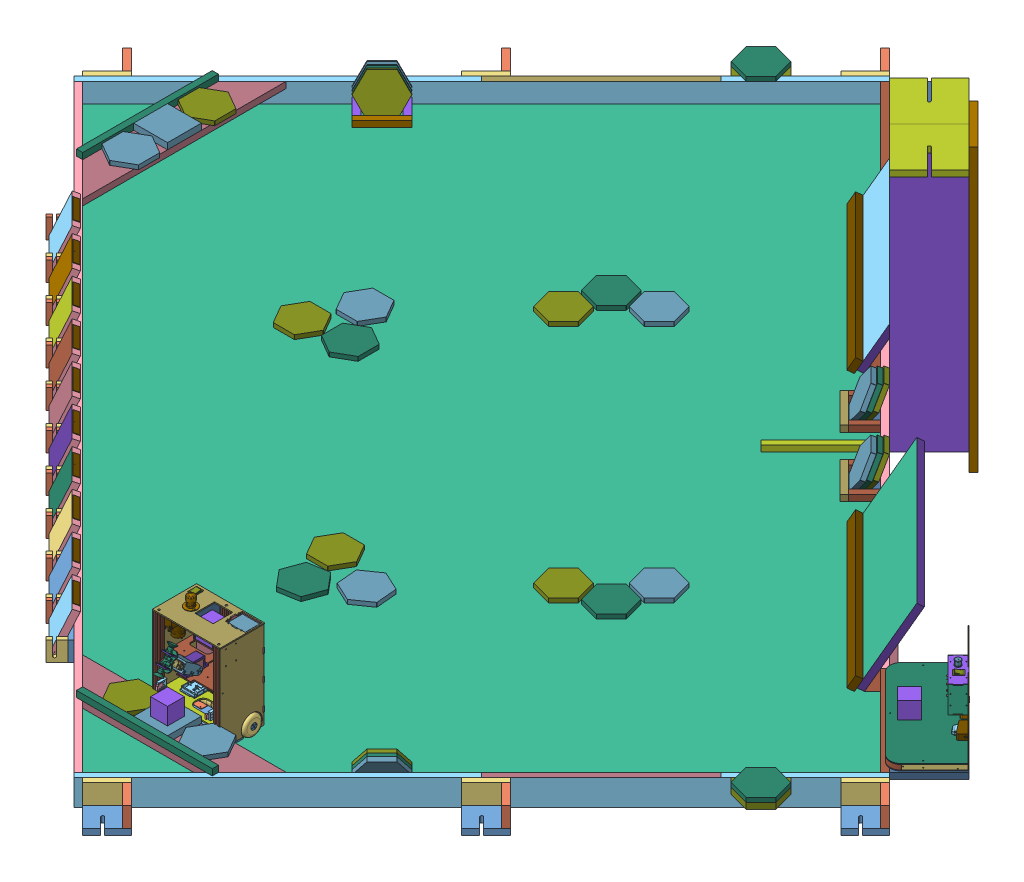
SolidWorks assembly conception_final_robot_autonome, configuration Default. Lengths in mm.
Overall size (3970.07 1029.4 3970.11).
442 component instances, 151 part files, 123 mates.
Components (placement in the parent):
- robot_sghyr-1: robot_sghyr [Default] at (76.8159 -4.9036 482.9829) x (0 0 1) z (0 1 0) size (182.75 247 90.25) (flexible)
  - base_robot_sghyr-1: base_robot_sghyr [Default] at (64.264 97.0127 214.7631) size (170 240 5)
  - 37 mm DC Geared Motor Mounting Bracket-1: 37 mm DC Geared Motor Mounting Bracket [Default] at (24.264 177.0127 247.7631) x (0 -1 0) z (-1 0 0) size (41 48 40)
  - pololu-37D-encoder-1: pololu-37D-encoder [Default] at (24.264 151.2127 247.7631) x (0 0 -1) z (0 1 0) size (36.8 36.8 92.61)
  - Robot2015_support bille porteuse-1: Robot2015_support bille porteuse [Défaut] at (126.764 97.0127 219.7631) x (-0.866025 -0.5 0) z (-0.5 0.866025 0) size (49.64 16.2 45)
  - 37 mm DC Geared Motor Mounting Bracket-3: 37 mm DC Geared Motor Mounting Bracket [Default] at (24.264 17.0127 247.7631) x (0 1 0) z (1 0 0) size (41 48 40)
  - pololu-37D-encoder-4: pololu-37D-encoder [Default] at (24.264 42.8127 247.7631) x (0 0 -1) z (0 -1 0) size (36.8 36.8 92.61)
  - Arduino Mega 2560.step-1: Arduino Mega 2560.step [Default] at (36.414 47.7209 283.4141) x (-1 0 0) z (0 0 -1) size (107.95 53.42 12.95)
  - Roulement_d3xd10xe4-1: Roulement_d3xd10xe4 [Défaut] at (146.264 -19.9873 225.0631) x (0 0 1) z (-1 0 0) size (5 13 13)
  - etage electronique-1: etage electronique [Default] at (64.264 97.0127 277.7631) x (0 -1 0) z (0 0 1) size (232 153 4)
  - XL4016E1 8A Buck Converter.STEP-1: XL4016E1 8A Buck Converter.STEP [Default] at (36.914 174.7627 281.7631) x (1 0 0) z (0 -1 0) size (65.3 28.6 46.4)
    - 8A Buck Converter PCB.STEP-1: 8A Buck Converter PCB.STEP [Default] at origin size (65.3 1.67 36.5)
    - Heat Exchanger.STEP-1: Heat Exchanger.STEP [Default] at (0 1.65 23.2) size (46 25.1 10.55)
    - Heat Exchanger.STEP-2: Heat Exchanger.STEP [Default] at (0 1.65 -23.2) x (-1 0 0) z (0 0 -1) size (46 25.1 10.55)
    - LargeGreen1000uF 35V Electrolytic Capacitor.STEP-1: LargeGreen1000uF 35V Electrolytic Capacitor.STEP [Default] at (-17.6782 1.65 7.8366) x (0 0 -1) z (1 0 0) size (9.9 26.01 9.9)
    - LargeGreen1000uF 35V Electrolytic Capacitor.STEP-2: LargeGreen1000uF 35V Electrolytic Capacitor.STEP [Default] at (-8.0317 1.65 5.0694) x (0 0 -1) z (1 0 0) size (9.9 26.01 9.9)
    - LargeGreen470uF 35V Electrolytic Capacitor.STEP-1: LargeGreen470uF 35V Electrolytic Capacitor.STEP [Default] at (-17.6617 1.65 -7.7514) x (0 0 1) z (-1 0 0) size (9.9 26.01 9.9)
    - LargeGreen470uF 35V Electrolytic Capacitor.STEP-2: LargeGreen470uF 35V Electrolytic Capacitor.STEP [Default] at (-7.9869 1.65 -5.0151) x (0 0 1) z (-1 0 0) size (9.9 26.01 9.9)
    - Screw Terminal x2.STEP-1: Screw Terminal x2.STEP [Default] at (-9.5 0 12.7839) x (-1 0 0) z (0 0 -1) size (7.95 12.9 10)
    - Screw Terminal x2.STEP-2: Screw Terminal x2.STEP [Default] at (-9.5 0 2.7839) x (-1 0 0) z (0 0 -1) size (7.95 12.9 10)
    - TrimmerW103.STEP-1: TrimmerW103.STEP [Default] at (32.65 6.9 -4.9563) x (0 0 1) z (-1 0 0) size (9.5 15.15 4.8)
    - TrimmerW103.STEP-2: TrimmerW103.STEP [Default] at (32.65 6.9 5.0581) x (0 0 1) z (-1 0 0) size (9.5 15.15 4.8)
    - whiteLEDShortLeed.STEP-1: whiteLEDShortLeed.STEP [Default] at (-13.9989 2.65 -0.1564) x (-1 0 0) z (0 0 -1) size (3.4 13.35 3.4)
    - Schottky Diode 20A 45V STPS2045CT.STEP-1: Schottky Diode 20A 45V STPS2045CT.STEP [Default] at (-0.0419 13.7002 12.65) x (-0.999962 0.008727 0) z (-0.008727 -0.999962 0) size (10.22 3.95 22.6)
    - XL4016E1 8A Voltage Regulator.STEP-1: XL4016E1 8A Voltage Regulator.STEP [Default] at (0 13.7 -12.65) x (1 0 0) z (0 -1 0) size (10.22 3.95 22.6)
    - Coil for Convertor.STEP-1: Coil for Convertor.STEP [Default] at (14.3115 2.9157 0.0112) size (27.99 14.39 26.86)
    - Small Plastic Washer.STEP-1: Small Plastic Washer.STEP [Default] at (0 18.5 -11.95) x (1 0 0) z (0 -1 0) size (6.1 1 6.1)
    - Small Plastic Washer.STEP-2: Small Plastic Washer.STEP [Default] at (0 18.5 10.95) x (1 0 0) z (0 -1 0) size (6.1 1 6.1)
    - pan head cross recess screw_iso_ISO 7045 - M3 x 8 - Z - 8S.STEP-1: pan head cross recess screw_iso_ISO 7045 - M3 x 8 - Z - 8S.STEP [Default] at (0 18.5 -8.55) x (0 0 -1) z (0.923728 0.383049 0) size (10.36 5.6 5.6)
    - pan head cross recess screw_iso_ISO 7045 - M3 x 8 - Z - 8S.STEP-2: pan head cross recess screw_iso_ISO 7045 - M3 x 8 - Z - 8S.STEP [Default] at (0 18.5 8.55) x (0 0 1) z (-1 0 0) size (10.36 5.6 5.6)
    - 1.7mmSmdCeramicCapacitorbrown.STEP-1: 1.7mmSmdCeramicCapacitorbrown.STEP [Default] at (2.849 0.0574 -8.3522) x (-1 0 0) z (0 0 1) size (2.02 0.49 1.04)
    - smdChip8pin.STEP-1: smdChip8pin.STEP [Default] at (19.9049 -0.725 7.6791) x (1 0 0) z (0 0 -1) size (7.3 1.22 4.5)
    - tinyVoltageRegulator.STEP-1: tinyVoltageRegulator.STEP [Default] at (13.3487 0 4.1964) x (-1 0 0) z (0 0 1) size (2.75 0.7 2.1)
    - tinyVoltageRegulator.STEP-2: tinyVoltageRegulator.STEP [Default] at (20.3011 0 11.2685) x (0.999962 0 0.008727) z (0.008727 0 -0.999962) size (2.75 0.7 2.1)
    - TinyVoltageRegulatorAMS1112.STEP-1: TinyVoltageRegulatorAMS1112.STEP [Default] at (15.0739 0.203 -4.8321) x (0 0 -1) z (-1 0 0) size (4.07 1.22 4.96)
    - tinySMDResistor222.STEP-1: tinySMDResistor222.STEP [Default] at (21.8501 0.1177 -6.1765) x (0 0 -1) z (-1 0 0) size (1.52 0.38 0.79)
    - tinySMDResistor.STEP-1: tinySMDResistor.STEP [Default] at (19.9225 0.1177 -6.1853) x (0 0 -1) z (-1 0 0) size (1.52 0.37 0.79)
    - 1.7mmSmdCeramicCapacitorbrown.STEP-2: 1.7mmSmdCeramicCapacitorbrown.STEP [Default] at (24.1073 0.0574 -6.3061) x (0 0 -1) z (-1 0 0) size (2.02 0.49 1.04)
    - 1.7mmSmdCeramicCapacitorbrown.STEP-3: 1.7mmSmdCeramicCapacitorbrown.STEP [Default] at (16.3262 0.0574 0.9562) x (0 0 -1) z (-1 0 0) size (2.02 0.49 1.04)
    - 1.7mmSmdCeramicCapacitorbrown.STEP-4: 1.7mmSmdCeramicCapacitorbrown.STEP [Default] at (18.1093 0.0574 0.9562) x (0 0 -1) z (-1 0 0) size (2.02 0.49 1.04)
    - tinySMDResistor.STEP-2: tinySMDResistor.STEP [Default] at (19.9874 0.1177 1.1419) x (0 0 -1) z (-1 0 0) size (1.52 0.37 0.79)
    - tinySMDResistor.STEP-3: tinySMDResistor.STEP [Default] at (21.6733 0.1177 1.1419) x (0 0 -1) z (-1 0 0) size (1.52 0.37 0.79)
    - tinySMDResistor.STEP-4: tinySMDResistor.STEP [Default] at (23.3916 0.1177 1.1419) x (0 0 -1) z (-1 0 0) size (1.52 0.37 0.79)
    - 1.7mmSmdCeramicCapacitorbrown.STEP-5: 1.7mmSmdCeramicCapacitorbrown.STEP [Default] at (25.4211 0.0574 4.0139) x (0 0 -1) z (-1 0 0) size (2.02 0.49 1.04)
    - 1.7mmSmdCeramicCapacitorbrown.STEP-6: 1.7mmSmdCeramicCapacitorbrown.STEP [Default] at (27.3088 0.0574 4.0139) x (0 0 -1) z (-1 0 0) size (2.02 0.49 1.04)
    - 1.7mmSmdCeramicCapacitorbrown.STEP-7: 1.7mmSmdCeramicCapacitorbrown.STEP [Default] at (23.1777 0.0574 11.1322) x (0 0 -1) z (-1 0 0) size (2.02 0.49 1.04)
    - 1.7mmSmdCeramicCapacitorbrown.STEP-8: 1.7mmSmdCeramicCapacitorbrown.STEP [Default] at (20.6839 0.0574 9.112) x (-0.999962 0 -0.008727) z (-0.008727 0 0.999962) size (2.02 0.49 1.04)
    - tinySMDResistor.STEP-5: tinySMDResistor.STEP [Default] at (17.7351 0.1177 11.3427) x (0 0 -1) z (-1 0 0) size (1.52 0.37 0.79)
    - tinySMDResistor.STEP-6: tinySMDResistor.STEP [Default] at (16.0827 0.1177 11.3427) x (0 0 -1) z (-1 0 0) size (1.52 0.37 0.79)
    - tinySMDResistor.STEP-7: tinySMDResistor.STEP [Default] at (16.906 0.1177 9.0199) x (-0.999962 0 -0.008727) z (-0.008727 0 0.999962) size (1.52 0.37 0.79)
    - tinySMDResistor.STEP-8: tinySMDResistor.STEP [Default] at (25.3907 0.1177 9.8144) x (-0.999962 0 -0.008727) z (-0.008727 0 0.999962) size (1.52 0.37 0.79)
    - R010 Resistor SMD.STEP-1: R010 Resistor SMD.STEP [Default] at (-19.919 0 5.2469) x (0 0 -1) z (-1 0 0) size (6.7 0.52 3.1)
    - solder.STEP-1: solder.STEP [Default] at (-27.65 0 -7.4411) x (-0.837169 0 -0.546944) z (-0.546944 0 0.837169) size (1.17 0.65 1.17)
    - solder.STEP-2: solder.STEP [Default] at (-27.65 0 -2.711) x (-0.837169 0 -0.546944) z (-0.546944 0 0.837169) size (1.17 0.65 1.17)
    - solder.STEP-3: solder.STEP [Default] at (-27.65 0 2.537) x (-0.837169 0 -0.546944) z (-0.546944 0 0.837169) size (1.17 0.65 1.17)
    - solder.STEP-4: solder.STEP [Default] at (-27.65 0 7.3016) x (-0.837169 0 -0.546944) z (-0.546944 0 0.837169) size (1.17 0.65 1.17)
    - solder1.8.STEP-1: solder1.8.STEP [Default] at (-20.8987 0 -15.5519) x (-0.837169 0 -0.546944) z (-0.546944 0 0.837169) size (1.8 0.65 1.8)
    - solder1.8.STEP-2: solder1.8.STEP [Default] at (20.8325 0 -15.5519) x (-0.837169 0 -0.546944) z (-0.546944 0 0.837169) size (1.8 0.65 1.8)
    - solder1.8.STEP-3: solder1.8.STEP [Default] at (20.8325 0 15.5391) x (-0.837169 0 -0.546944) z (-0.546944 0 0.837169) size (1.8 0.65 1.8)
    - solder1.8.STEP-4: solder1.8.STEP [Default] at (-20.8987 0 15.5391) x (-0.837169 0 -0.546944) z (-0.546944 0 0.837169) size (1.8 0.65 1.8)
    - solder.STEP-5: solder.STEP [Default] at (30.4698 0 7.6228) x (-0.837169 0 -0.546944) z (-0.546944 0 0.837169) size (1.17 0.65 1.17)
    - solder.STEP-6: solder.STEP [Default] at (30.4698 0 2.537) x (-0.837169 0 -0.546944) z (-0.546944 0 0.837169) size (1.17 0.65 1.17)
    - solder.STEP-7: solder.STEP [Default] at (30.4698 0 -2.454) x (-0.837169 0 -0.546944) z (-0.546944 0 0.837169) size (1.17 0.65 1.17)
    - solder.STEP-8: solder.STEP [Default] at (30.4698 0 -7.4732) x (-0.837169 0 -0.546944) z (-0.546944 0 0.837169) size (1.17 0.65 1.17)
    - solder.STEP-9: solder.STEP [Default] at (30.4698 0 -4.9355) x (-0.837169 0 -0.546944) z (-0.546944 0 0.837169) size (1.17 0.65 1.17)
    - solder.STEP-10: solder.STEP [Default] at (30.4698 0 5.0529) x (-0.837169 0 -0.546944) z (-0.546944 0 0.837169) size (1.17 0.65 1.17)
    - solder1.8.STEP-5: solder1.8.STEP [Default] at (1.0959 0 2.1506) x (-0.837169 0 -0.546944) z (-0.546944 0 0.837169) size (1.8 0.65 1.8)
    - solder1.8.STEP-6: solder1.8.STEP [Default] at (8.9457 0 2.3519) x (-0.837169 0 -0.546944) z (-0.546944 0 0.837169) size (1.8 0.65 1.8)
    - solder.STEP-11: solder.STEP [Default] at (-3.9931 0 -10.2017) x (-0.837169 0 -0.546944) z (-0.546944 0 0.837169) size (1.17 0.65 1.17)
    - solder.STEP-12: solder.STEP [Default] at (-1.9931 0 -10.2017) x (-0.837169 0 -0.546944) z (-0.546944 0 0.837169) size (1.17 0.65 1.17)
    - solder.STEP-13: solder.STEP [Default] at (0.0069 0 -10.2017) x (-0.837169 0 -0.546944) z (-0.546944 0 0.837169) size (1.17 0.65 1.17)
    - solder.STEP-14: solder.STEP [Default] at (2.0069 0 -10.2017) x (-0.837169 0 -0.546944) z (-0.546944 0 0.837169) size (1.17 0.65 1.17)
    - solder.STEP-15: solder.STEP [Default] at (4.0069 0 -10.2017) x (-0.837169 0 -0.546944) z (-0.546944 0 0.837169) size (1.17 0.65 1.17)
    - solder.STEP-16: solder.STEP [Default] at (-2.7433 0 10.0764) x (-0.873283 0 -0.487214) z (-0.487214 0 0.873283) size (1.17 0.65 1.17)
    - solder.STEP-17: solder.STEP [Default] at (-0.2033 0 10.0764) x (-0.873283 0 -0.487214) z (-0.487214 0 0.873283) size (1.17 0.65 1.17)
    - solder.STEP-18: solder.STEP [Default] at (2.3367 0 10.0764) x (-0.873283 0 -0.487214) z (-0.487214 0 0.873283) size (1.17 0.65 1.17)
    - solder.STEP-19: solder.STEP [Default] at (-8.0296 0 7.8897) x (-0.873283 0 -0.487214) z (-0.487214 0 0.873283) size (1.17 0.65 1.17)
    - solder.STEP-20: solder.STEP [Default] at (-8.0296 0 2.259) x (-0.873283 0 -0.487214) z (-0.487214 0 0.873283) size (1.17 0.65 1.17)
    - solder.STEP-21: solder.STEP [Default] at (-8.0296 0 -2.2341) x (-0.873283 0 -0.487214) z (-0.487214 0 0.873283) size (1.17 0.65 1.17)
    - solder.STEP-22: solder.STEP [Default] at (-8.0296 0 -7.8634) x (-0.873283 0 -0.487214) z (-0.487214 0 0.873283) size (1.17 0.65 1.17)
    - solder.STEP-23: solder.STEP [Default] at (-17.6872 0 -10.549) x (-0.873283 0 -0.487214) z (-0.487214 0 0.873283) size (1.17 0.65 1.17)
    - solder.STEP-24: solder.STEP [Default] at (-17.6872 0 -4.9388) x (-0.873283 0 -0.487214) z (-0.487214 0 0.873283) size (1.17 0.65 1.17)
    - solder.STEP-25: solder.STEP [Default] at (-17.6872 0 10.6333) x (-0.873283 0 -0.487214) z (-0.487214 0 0.873283) size (1.17 0.65 1.17)
    - solder.STEP-26: solder.STEP [Default] at (-17.6872 0 5.0231) x (-0.873283 0 -0.487214) z (-0.487214 0 0.873283) size (1.17 0.65 1.17)
    - solder.STEP-27: solder.STEP [Default] at (-15.2798 0 -0.193) x (-0.873283 0 -0.487214) z (-0.487214 0 0.873283) size (1.17 0.65 1.17)
    - solder.STEP-28: solder.STEP [Default] at (-12.7921 0 -0.193) x (-0.873283 0 -0.487214) z (-0.487214 0 0.873283) size (1.17 0.65 1.17)
  - Roulement_d3xd10xe4-3: Roulement_d3xd10xe4 [Défaut] at (146.264 214.0127 225.0631) x (0 0 1) z (1 0 0) size (5 13 13)
- étage 3-1: étage 3 [Default] at (169.8286 379.2835 544.2469) x (0 0 1) z (-1 0 0) size (162 4 232)
- ##Servo_MG_996R-3: ##Servo_MG_996R [Default] at (167.7867 418.7449 625.8548) x (-1 0 0) z (0 0.826818 -0.562469) size (53.6 45.5 20)
- Servo-1: Servo [Défaut] at (182.7867 399.2835 587.7469) x (0 -1 0) z (-1 0 0) size (32 43 41.5)
- bras_replique-1: bras_replique [Default] at (141.7867 399.2835 597.2469) x (0 0.562469 0.826818) z (1 0 0) size (77.5 32 70)
- SUPPORT VENTOUSE-1: SUPPORT VENTOUSE [Default] at (157.7867 442.9311 661.408) x (0 0.826818 -0.562469) z (0 0.562469 0.826818) size (60 44.83 4)
- Access_HS-645_BrasRondPetitModele-1: Access_HS-645_BrasRondPetitModele [Défaut] at (157.7867 442.6499 660.9946) x (1 0 0) z (0 -0.826818 0.562469) size (24 5 24)
- support servo kbyr-1: support servo kbyr [Default] at (181.5367 383.2835 548.2469) x (0 0 1) z (-1 0 0) size (79 38 30)
- PompeVide-AirpoD2028B-12vdc-1: PompeVide-AirpoD2028B-12vdc [Défaut] at (270.3286 514.8594 552.1469) x (1 0 0) z (0 -1 0) size (38.6 62.4 92)
- TABLE_2021.step-1: TABLE_2021.step [Default] at (-533.2781 201.1947 -2548.6626) x (0.707107 0 0.707107) z (0 1 0) size (3306.25 2336 1029.4)
  - BaseTable.step-1: BaseTable.step [Default] at (0 0 -22) x (1 0 0) z (0 -1 0) size (3288 1022 2266)
    - Edge Beacon Right.step-1: Edge Beacon Right.step [Default] at (-884.0915 354.4211 0) x (1 0 0) z (0 1 0) size (122 122 92)
      - EdgeBeacons_Base.step-1: EdgeBeacons_Base.step [Default] at (3967.0915 -989 -332.4211) x (0 -1 0) z (1 0 0) size (122 22 122)
      - EdgeBeacons_SmallBorder.step-1: EdgeBeacons_SmallBorder.step [Default] at (4028.0915 -950 -332.4211) x (0 1 0) z (1 0 0) size (22 70 100)
      - EdgeBeacons_LargeBorder.step-1: EdgeBeacons_LargeBorder.step [Default] at (3906.0915 -1050 -332.4211) x (1 0 0) z (0 -1 0) size (22 70 122)
    - Edge Beacon Left.step-1: Edge Beacon Left.step [Default] at (-1609.4995 44.4467 0) x (1 0 0) z (0 1 0) size (122 122 92)
      - EdgeBeacons_Base.step-1: EdgeBeacons_Base.step [Default] at (1526.4995 -39 -44.4467) x (0 -1 0) z (-1 0 0) size (122 22 122)
      - EdgeBeacons_LargeBorder.step-1: EdgeBeacons_LargeBorder.step [Default] at (1565.4995 -100 -22.4467) x (1 0 0) z (0 -1 0) size (22 70 122)
      - EdgeBeacons_SmallBorder.step-1: EdgeBeacons_SmallBorder.step [Default] at (1465.4995 22 -22.4467) x (0 -1 0) z (-1 0 0) size (22 70 100)
    - Edge Beacon Right_1.step-1: Edge Beacon Right_1.step [Default] at (-884.0915 354.4211 0) x (1 0 0) z (0 1 0) size (122 122 92)
      - EdgeBeacons_Base.step-1: EdgeBeacons_Base.step [Default] at (3967.0915 -39 -332.4211) x (0 -1 0) z (1 0 0) size (122 22 122)
      - EdgeBeacons_SmallBorder.step-1: EdgeBeacons_SmallBorder.step [Default] at (4028.0915 0 -332.4211) x (0 1 0) z (1 0 0) size (22 70 100)
      - EdgeBeacons_LargeBorder.step-1: EdgeBeacons_LargeBorder.step [Default] at (3906.0915 -100 -332.4211) x (1 0 0) z (0 -1 0) size (22 70 122)
    - Edge Beacon Right_2.step-1: Edge Beacon Right_2.step [Default] at (-1546.4323 1056.5508 0) x (1 0 0) z (0 1 0) size (122 122 92)
      - EdgeBeacons_Base.step-1: EdgeBeacons_Base.step [Default] at (4629.4323 -1939 -1034.5508) x (0 -1 0) z (1 0 0) size (122 22 122)
      - EdgeBeacons_SmallBorder.step-1: EdgeBeacons_SmallBorder.step [Default] at (4690.4323 -1900 -1034.5508) x (0 1 0) z (1 0 0) size (22 70 100)
      - EdgeBeacons_LargeBorder.step-1: EdgeBeacons_LargeBorder.step [Default] at (4568.4323 -2000 -1034.5508) x (1 0 0) z (0 -1 0) size (22 70 122)
    - Edge Beacon Left_1.step-1: Edge Beacon Left_1.step [Default] at (-933.7648 1396.3534 0) x (1 0 0) z (0 1 0) size (122 122 92)
      - EdgeBeacons_Base.step-1: EdgeBeacons_Base.step [Default] at (850.7648 -1939 -1396.3534) x (0 -1 0) z (-1 0 0) size (122 22 122)
      - EdgeBeacons_LargeBorder.step-1: EdgeBeacons_LargeBorder.step [Default] at (889.7648 -2000 -1374.3534) x (1 0 0) z (0 -1 0) size (22 70 122)
      - EdgeBeacons_SmallBorder.step-1: EdgeBeacons_SmallBorder.step [Default] at (789.7648 -1878 -1374.3534) x (0 -1 0) z (-1 0 0) size (22 70 100)
    - Edge Beacon Left_2.step-1: Edge Beacon Left_2.step [Default] at (-2304.4911 1279.1137 0) x (1 0 0) z (0 1 0) size (122 122 92)
      - EdgeBeacons_Base.step-1: EdgeBeacons_Base.step [Default] at (2221.4911 -989 -1279.1137) x (0 -1 0) z (-1 0 0) size (122 22 122)
      - EdgeBeacons_LargeBorder.step-1: EdgeBeacons_LargeBorder.step [Default] at (2260.4911 -1050 -1257.1137) x (1 0 0) z (0 -1 0) size (22 70 122)
      - EdgeBeacons_SmallBorder.step-1: EdgeBeacons_SmallBorder.step [Default] at (2160.4911 -928 -1257.1137) x (0 -1 0) z (-1 0 0) size (22 70 100)
    - BorderLong.step-1: BorderLong.step [Default] at (0 0 -22) size (3000 92 22)
    - BorderLong.step-2: BorderLong.step [Default] at (3000 0 2022) x (-1 0 0) z (0 0 -1) size (3000 92 22)
    - BorderSmall.step-1: BorderSmall.step [Default] at (-22 0 2022) x (0 0 -1) z (1 0 0) size (2044 92 22)
    - BorderSmall.step-2: BorderSmall.step [Default] at (3022 0 -22) x (0 0 1) z (-1 0 0) size (2044 92 22)
    - Ground.step-1: Ground.step [Default] at origin size (3000 22 2000)
    - MiddleBeaconTop.step-1: MiddleBeaconTop.step [Default] at (1500 22 -122) size (400 22 200)
    - MiddleBeaconVertSupport1.step-1: MiddleBeaconVertSupport1.step [Default] at (1500 22 -22) x (0 0 1) z (-1 0 0) size (200 978 22)
    - MiddleBeaconVertSupport2.step-1: MiddleBeaconVertSupport2.step [Default] at (1600 22 -233) size (200 1000 22)
    - ExperimentZone.step-1: ExperimentZone.step [Default] at (225 92 -22) size (450 22 200)
    - ExperimentZone.step-2: ExperimentZone.step [Default] at (2775 92 -22) size (450 22 200)
    - PaintExperience.step-1: PaintExperience.step [Default] at (0 92 -22) size (450 0.1 22)
    - PaintExperience.step-2: PaintExperience.step [Default] at (2550 92 -22) size (450 0.1 22)
    - BaseTable-0.step-1: BaseTable-0.step [Default] at origin size (22 0.1 600)
    - BaseTable-1.step-1: BaseTable-1.step [Default] at origin size (22 0.1 600)
  - Echantillons.step-1: Echantillons.step [Default] at origin size (3292.15 1762.13 85)
    - EchantillonBleu.step-1: EchantillonBleu.step [Default] at (900 -555 0) x (0.5 0.866025 0) z (0 0 1) size (129.9 149.69 15)
    - EchantillonBleu.step-2: EchantillonBleu.step [Default] at (892.3031 -1292.3031 15) x (0.965926 0.258819 0) z (0 0 -1) size (129.9 149.69 15)
    - EchantillonBleu.step-3: EchantillonBleu.step [Default] at (2100 -555 0) x (0.5 0.866025 0) z (0 0 1) size (129.9 149.69 15)
    - EchantillonBleu.step-4: EchantillonBleu.step [Default] at (2113.9218 -1288.3769 15) x (0.34202 -0.939693 0) z (0 0 -1) size (129.9 149.69 15)
    - EchantillonVert.step-1: EchantillonVert.step [Default] at (2085.0581 -1446.2787 15) x (0.906308 0.422618 0) z (0 0 -1) size (129.9 149.69 15)
    - EchantillonRouge.step-1: EchantillonRouge.step [Default] at (1954.3221 -1366.4789 15) x (0.258819 0.965926 0) z (0 0 -1) size (129.9 149.69 15)
    - EchantillonVert.step-2: EchantillonVert.step [Default] at (830 -675 0) x (0.5 0.866025 0) z (0 0 1) size (129.9 149.69 15)
    - EchantillonRouge.step-2: EchantillonRouge.step [Default] at (900 -795 0) x (0.5 0.866025 0) z (0 0 1) size (129.9 149.69 15)
    - EchantillonVert.step-3: EchantillonVert.step [Default] at (2170 -675 0) x (0.5 0.866025 0) z (0 0 1) size (129.9 149.69 15)
    - EchantillonRouge.step-3: EchantillonRouge.step [Default] at (2100 -795 0) x (0.5 0.866025 0) z (0 0 1) size (129.9 149.69 15)
    - EchantillonVert.step-4: EchantillonVert.step [Default] at (1044.2641 -1329.1257 15) x (0.965926 -0.258819 0) z (0 0 -1) size (129.9 149.69 15)
    - EchantillonRouge.step-4: EchantillonRouge.step [Default] at (950 -1450 15) x (0.965926 0.258819 0) z (0 0 -1) size (129.9 149.69 15)
    - EchantillonBleu.step-5: EchantillonBleu.step [Default] at (311.5685 -1879.3503 70) x (0.258819 -0.965926 0) z (0 0 1) size (129.9 149.69 15)
    - EchantillonRouge.step-5: EchantillonRouge.step [Default] at (120.6497 -1688.4315 70) x (-0.258819 0.965926 0) z (0 0 1) size (129.9 149.69 15)
    - EchantillonBleu.step-6: EchantillonBleu.step [Default] at (2879.3503 -1688.4315 70) x (0.965926 0.258819 0) z (0 0 1) size (129.9 149.69 15)
    - EchantillonRouge.step-6: EchantillonRouge.step [Default] at (2688.4315 -1879.3503 70) x (-0.965926 -0.258819 0) z (0 0 1) size (129.9 149.69 15)
    - EchantillonVert.step-5: EchantillonVert.step [Default] at (-64.9519 -300 70) x (-0.5 0.866025 0) z (0 0 1) size (129.9 149.69 15)
    - EchantillonVert.step-6: EchantillonVert.step [Default] at (3064.9519 -300 70) size (129.9 149.69 15)
  - Frises.step-1: Frises.step [Default] at origin size (2100 194.46 292.81)
    - FriseJaune.step-1: FriseJaune.step [Default] at (810 0 0) x (0 -1 0) z (0 0 1) size (194.46 720 292.81)
      - Frise.step-1: Frise.step [Default] at origin size (194.46 720 292.81)
        - FRISE_2.step-1: FRISE_2.step [Default] at origin size (169.05 720 270.81)
        - BORDURE.step-1: BORDURE.step [Default] at origin size (41.05 720 49.11)
        - TRIANGLE_GAUCHE.step-1: TRIANGLE_GAUCHE.step [Default] at origin size (40.41 22 70)
        - TRIANGLE_DROIT.step-1: TRIANGLE_DROIT.step [Default] at origin size (40.41 22 70)
        - TRIANGLE_CENTRE.step-1: TRIANGLE_CENTRE.step [Default] at origin size (40.41 22 70)
        - TaquetArriere.step-1: TaquetArriere.step [Default] at origin size (22 22 168.21)
        - TaquetArriere.step-2: TaquetArriere.step [Default] at (0 698 0) size (22 22 168.21)
        - TaquetArriere.step-3: TaquetArriere.step [Default] at (0 349 0) size (22 22 168.21)
      - FriseJaune-2.step-1: FriseJaune-2.step [Default] at origin size (150.01 720 259.81)
    - FriseViolet.step-1: FriseViolet.step [Default] at (2190 0 0) x (0 -1 0) z (0 0 1) size (194.46 720 292.81)
      - Frise_1.step-1: Frise_1.step [Default] at origin size (194.46 720 292.81)
        - FRISE_2.step-1: FRISE_2.step [Default] at origin size (169.05 720 270.81)
        - BORDURE.step-1: BORDURE.step [Default] at origin size (41.05 720 49.11)
        - TRIANGLE_GAUCHE.step-1: TRIANGLE_GAUCHE.step [Default] at origin size (40.41 22 70)
        - TRIANGLE_DROIT.step-1: TRIANGLE_DROIT.step [Default] at origin size (40.41 22 70)
        - TRIANGLE_CENTRE.step-1: TRIANGLE_CENTRE.step [Default] at origin size (40.41 22 70)
        - TaquetArriere.step-1: TaquetArriere.step [Default] at origin size (22 22 168.21)
        - TaquetArriere.step-2: TaquetArriere.step [Default] at (0 698 0) size (22 22 168.21)
        - TaquetArriere.step-3: TaquetArriere.step [Default] at (0 349 0) size (22 22 168.21)
      - FriseViolet-3.step-1: FriseViolet-3.step [Default] at origin size (150.01 720 259.81)
  - Distributeurs.step-1: Distributeurs.step [Default] at origin size (3259.81 2051.07 183.14)
    - Distributeur 2 Side.step-1: Distributeur 2 Side.step [Default] at (11 -1250 0) x (0 1 0) z (1 0 0) size (187.35 183.14 137.52)
      - TasseauBordure.step-1: TasseauBordure.step [Default] at origin size (106 22 22)
      - TasseauCote.step-1: TasseauCote.step [Default] at (-64 0 29) size (22 22 80)
      - TasseauCote.step-2: TasseauCote.step [Default] at (64 0 29) size (22 22 80)
      - TasseauAvant.step-1: TasseauAvant.step [Default] at (0 0 80) size (150 22 22)
      - EchantillonBleu.step-1: EchantillonBleu.step [Default] at (0 59.0455 -5.9792) x (0.866025 0.454532 -0.208327) z (0 0.416655 0.909065) size (129.9 149.69 15)
      - EchantillonVert.step-1: EchantillonVert.step [Default] at (0 59.0455 10.5213) x (0.866025 0.454532 -0.208327) z (0 0.416655 0.909065) size (129.9 149.69 15)
      - EchantillonRouge.step-1: EchantillonRouge.step [Default] at (0 59.0455 27.0218) x (0.866025 0.454532 -0.208327) z (0 0.416655 0.909065) size (129.9 149.69 15)
    - Distributeur 2 Side_1.step-1: Distributeur 2 Side_1.step [Default] at (2989 -1250 0) x (0 -1 0) z (-1 0 0) size (187.35 183.14 137.52)
      - TasseauBordure.step-1: TasseauBordure.step [Default] at origin size (106 22 22)
      - TasseauCote.step-1: TasseauCote.step [Default] at (-64 0 29) size (22 22 80)
      - TasseauCote.step-2: TasseauCote.step [Default] at (64 0 29) size (22 22 80)
      - TasseauAvant.step-1: TasseauAvant.step [Default] at (0 0 80) size (150 22 22)
      - EchantillonBleu.step-1: EchantillonBleu.step [Default] at (0 59.0455 -5.9792) x (0.866025 0.454532 -0.208327) z (0 0.416655 0.909065) size (129.9 149.69 15)
      - EchantillonVert.step-1: EchantillonVert.step [Default] at (0 59.0455 10.5213) x (0.866025 0.454532 -0.208327) z (0 0.416655 0.909065) size (129.9 149.69 15)
      - EchantillonRouge.step-1: EchantillonRouge.step [Default] at (0 59.0455 27.0218) x (0.866025 0.454532 -0.208327) z (0 0.416655 0.909065) size (129.9 149.69 15)
    - Distributeur 2 Top.step-1: Distributeur 2 Top.step [Default] at (1650 -11 0) x (1 0 0) z (0 -1 0) size (187.35 183.14 137.52)
      - TasseauBordure_1.step-1: TasseauBordure_1.step [Default] at origin size (106 22 22)
      - TasseauCote_1.step-1: TasseauCote_1.step [Default] at (-64 0 29) size (22 22 80)
      - TasseauCote_1.step-2: TasseauCote_1.step [Default] at (64 0 29) size (22 22 80)
      - TasseauAvant_1.step-1: TasseauAvant_1.step [Default] at (0 0 80) size (150 22 22)
      - EchantillonBleu.step-1: EchantillonBleu.step [Default] at (0 59.0455 27.0218) x (0.866025 0.454532 -0.208327) z (0 0.416655 0.909065) size (129.9 149.69 15)
      - EchantillonRouge.step-1: EchantillonRouge.step [Default] at (0 59.0455 -5.9792) x (0.866025 0.454532 -0.208327) z (0 0.416655 0.909065) size (129.9 149.69 15)
      - EchantillonVert.step-1: EchantillonVert.step [Default] at (0 59.0455 10.5213) x (0.866025 0.454532 -0.208327) z (0 0.416655 0.909065) size (129.9 149.69 15)
    - Distributeur 2 Top_1.step-1: Distributeur 2 Top_1.step [Default] at (1350 -11 0) x (1 0 0) z (0 -1 0) size (187.35 183.14 137.52)
      - TasseauBordure_1.step-1: TasseauBordure_1.step [Default] at origin size (106 22 22)
      - TasseauCote_1.step-1: TasseauCote_1.step [Default] at (-64 0 29) size (22 22 80)
      - TasseauCote_1.step-2: TasseauCote_1.step [Default] at (64 0 29) size (22 22 80)
      - TasseauAvant_1.step-1: TasseauAvant_1.step [Default] at (0 0 80) size (150 22 22)
      - EchantillonBleu.step-1: EchantillonBleu.step [Default] at (0 59.0455 27.0218) x (0.866025 0.454532 -0.208327) z (0 0.416655 0.909065) size (129.9 149.69 15)
      - EchantillonRouge.step-1: EchantillonRouge.step [Default] at (0 59.0455 -5.9792) x (0.866025 0.454532 -0.208327) z (0 0.416655 0.909065) size (129.9 149.69 15)
      - EchantillonVert.step-1: EchantillonVert.step [Default] at (0 59.0455 10.5213) x (0.866025 0.454532 -0.208327) z (0 0.416655 0.909065) size (129.9 149.69 15)
    - DistributeurCoin.step-1: DistributeurCoin.step [Default] at (0 -2000 175) size (525.56 525.56 44)
      - Taquet.step-1: Taquet.step [Default] at (0 0 -197) size (510 510 22)
      - SupportStatuette.step-1: SupportStatuette.step [Default] at (0 0 -197) size (169.71 169.71 22)
      - Taquet (1).step-1: Taquet (1).step [Default] at (0 0 -197) size (355.85 355.85 22)
    - DistributeurCoin_1.step-1: DistributeurCoin_1.step [Default] at (3000 -2000 300) x (0 1 0) z (0 0 1) size (525.56 525.56 44)
      - Taquet.step-1: Taquet.step [Default] at (0 0 -322) size (510 510 22)
      - SupportStatuette.step-1: SupportStatuette.step [Default] at (0 0 -322) size (169.71 169.71 22)
      - Taquet (1).step-1: Taquet (1).step [Default] at (0 0 -322) size (355.85 355.85 22)
    - DistributeurBordure.step-1: DistributeurBordure.step [Default] at (-200 -250 0) size (107.9 150 92)
      - Support (1).step-1: Support (1).step [Default] at (200 -50 -22) size (107.9 150 22)
      - Equerre.step-1: Equerre.step [Default] at (200 -50 -22) size (70 22 70)
    - DistributeurBordure_1.step-1: DistributeurBordure_1.step [Default] at (3250 -250 0) x (-1 0 0) z (0 0 1) size (107.9 150 92)
      - Support (1).step-1: Support (1).step [Default] at (250 50 -22) size (107.9 150 22)
      - Equerre.step-1: Equerre.step [Default] at (250 50 -22) size (70 22 70)
  - CarreFouille.step-1: CarreFouille.step [Default] at origin size (1850 85.95 153.3)
    - CarreFouilleTresorJaune.step-1: CarreFouilleTresorJaune.step [Default] at (667.5 -2000 0) x (0 -1 0) z (0 0 1) size (85.95 185 153.3)
      - CarreFouille_1.step-1: CarreFouille_1.step [Default] at (64.8942 -232.3942 0) size (85.94 185 153.3)
        - PCB_datation.step-1: PCB_datation.step [Default] at (0 0 158.7231) x (0 1 0) z (0 0 1) size (100 19.02 9.26)
          - PCB Component.step-1: PCB Component.step [Default] at (232.3942 48.7058 -10.7729) x (1 0 0) z (0 0.390731 0.920505) size (100 20 1.57)
            - Board.step-1: Board.step [Default] at origin size (100 20 1.57)
        - BASE.step-1: BASE.step [Default] at (-27.8942 232.3942 35) size (15 185 70)
        - LEFT_ARM.step-1: LEFT_ARM.step [Default] at (-27.8942 232.3942 35) size (55 15 70)
        - RIGHT_ARM.step-1: RIGHT_ARM.step [Default] at (-27.8942 232.3942 35) size (55 15 70)
        - SQUARE.step-1: SQUARE.step [Default] at (-31.092 232.3942 20.7181) x (0.920505 0 0.390731) z (-0.390731 0 0.920505) size (22 150 150)
      - CarreFouilleTresorJaune-4.step-1: CarreFouilleTresorJaune-4.step [Default] at origin size (58.62 150 138.08)
      - CarreFouilleTresorJaune-5.step-1: CarreFouilleTresorJaune-5.step [Default] at origin size (58.62 150 138.08)
    - CarreFouilleRadioactif.step-1: CarreFouilleRadioactif.step [Default] at (1037.5 -2000 0) x (0 -1 0) z (0 0 1) size (85.95 185 153.3)
      - CarreFouille_2.step-1: CarreFouille_2.step [Default] at (364.8942 -102.3942 0) size (85.94 185 153.3)
        - PCB_datation_1.step-1: PCB_datation_1.step [Default] at (0 0 158.7231) x (0 1 0) z (0 0 1) size (100 19.02 9.26)
          - PCB Component_1.step-1: PCB Component_1.step [Default] at (102.3942 348.7058 -10.7729) x (1 0 0) z (0 0.390731 0.920505) size (100 20 1.57)
            - Board.step-1: Board.step [Default] at origin size (100 20 1.57)
        - BASE.step-1: BASE.step [Default] at (-327.8942 102.3942 35) size (15 185 70)
        - LEFT_ARM.step-1: LEFT_ARM.step [Default] at (-327.8942 102.3942 35) size (55 15 70)
        - RIGHT_ARM.step-1: RIGHT_ARM.step [Default] at (-327.8942 102.3942 35) size (55 15 70)
        - SQUARE.step-1: SQUARE.step [Default] at (-331.092 102.3942 20.7181) x (0.920505 0 0.390731) z (-0.390731 0 0.920505) size (22 150 150)
      - CarreFouilleRadioactif-6.step-1: CarreFouilleRadioactif-6.step [Default] at origin size (58.62 150 138.08)
      - CarreFouilleRadioactif-7.step-1: CarreFouilleRadioactif-7.step [Default] at origin size (58.62 150 138.08)
    - CarreFouilleTresorJaune_1.step-1: CarreFouilleTresorJaune_1.step [Default] at (852.5 -2000 0) x (0 -1 0) z (0 0 1) size (85.95 185 153.3)
      - CarreFouille_3.step-1: CarreFouille_3.step [Default] at (264.8942 282.6058 0) size (85.94 185 153.3)
        - PCB_datation_2.step-1: PCB_datation_2.step [Default] at (0 0 158.7231) x (0 1 0) z (0 0 1) size (100 19.02 9.26)
          - PCB Component_2.step-1: PCB Component_2.step [Default] at (-282.6058 248.7058 -10.7729) x (1 0 0) z (0 0.390731 0.920505) size (100 20 1.57)
            - Board.step-1: Board.step [Default] at origin size (100 20 1.57)
        - BASE.step-1: BASE.step [Default] at (-227.8942 -282.6058 35) size (15 185 70)
        - LEFT_ARM.step-1: LEFT_ARM.step [Default] at (-227.8942 -282.6058 35) size (55 15 70)
        - RIGHT_ARM.step-1: RIGHT_ARM.step [Default] at (-227.8942 -282.6058 35) size (55 15 70)
        - SQUARE.step-1: SQUARE.step [Default] at (-231.092 -282.6058 20.7181) x (0.920505 0 0.390731) z (-0.390731 0 0.920505) size (22 150 150)
      - CarreFouilleTresorJaune_1-8.step-1: CarreFouilleTresorJaune_1-8.step [Default] at origin size (58.62 150 138.08)
      - CarreFouilleTresorJaune_1-9.step-1: CarreFouilleTresorJaune_1-9.step [Default] at origin size (58.62 150 138.08)
    - CarreFouilleTresorViolet.step-1: CarreFouilleTresorViolet.step [Default] at (1222.5 -2000 0) x (0 -1 0) z (0 0 1) size (85.95 185 153.3)
      - CarreFouille_4.step-1: CarreFouille_4.step [Default] at (464.8942 112.6058 0) size (85.94 185 153.3)
        - PCB_datation_3.step-1: PCB_datation_3.step [Default] at (0 0 158.7231) x (0 1 0) z (0 0 1) size (100 19.02 9.26)
          - PCB Component_3.step-1: PCB Component_3.step [Default] at (-112.6058 448.7058 -10.7729) x (1 0 0) z (0 0.390731 0.920505) size (100 20 1.57)
            - Board.step-1: Board.step [Default] at origin size (100 20 1.57)
        - BASE.step-1: BASE.step [Default] at (-427.8942 -112.6058 35) size (15 185 70)
        - LEFT_ARM.step-1: LEFT_ARM.step [Default] at (-427.8942 -112.6058 35) size (55 15 70)
        - RIGHT_ARM.step-1: RIGHT_ARM.step [Default] at (-427.8942 -112.6058 35) size (55 15 70)
        - SQUARE.step-1: SQUARE.step [Default] at (-431.092 -112.6058 20.7181) x (0.920505 0 0.390731) z (-0.390731 0 0.920505) size (22 150 150)
      - CarreFouilleTresorViolet-10.step-1: CarreFouilleTresorViolet-10.step [Default] at origin size (58.62 150 138.08)
      - CarreFouilleTresorViolet-11.step-1: CarreFouilleTresorViolet-11.step [Default] at origin size (58.62 150 138.08)
    - CarreFouilleTresorJaune_2.step-1: CarreFouilleTresorJaune_2.step [Default] at (1407.5 -2000 0) x (0 -1 0) z (0 0 1) size (85.95 185 153.3)
      - CarreFouille_5.step-1: CarreFouille_5.step [Default] at (464.8942 27.6058 0) size (85.94 185 153.3)
        - PCB_datation_4.step-1: PCB_datation_4.step [Default] at (0 0 158.7231) x (0 1 0) z (0 0 1) size (100 19.02 9.26)
          - PCB Component_4.step-1: PCB Component_4.step [Default] at (-27.6058 448.7058 -10.7729) x (1 0 0) z (0 0.390731 0.920505) size (100 20 1.57)
            - Board.step-1: Board.step [Default] at origin size (100 20 1.57)
        - BASE.step-1: BASE.step [Default] at (-427.8942 -27.6058 35) size (15 185 70)
        - LEFT_ARM.step-1: LEFT_ARM.step [Default] at (-427.8942 -27.6058 35) size (55 15 70)
        - RIGHT_ARM.step-1: RIGHT_ARM.step [Default] at (-427.8942 -27.6058 35) size (55 15 70)
        - SQUARE.step-1: SQUARE.step [Default] at (-431.092 -27.6058 20.7181) x (0.920505 0 0.390731) z (-0.390731 0 0.920505) size (22 150 150)
      - CarreFouilleTresorJaune_2-12.step-1: CarreFouilleTresorJaune_2-12.step [Default] at origin size (58.62 150 138.08)
      - CarreFouilleTresorJaune_2-13.step-1: CarreFouilleTresorJaune_2-13.step [Default] at origin size (58.62 150 138.08)
    - CarreFouilleTresorViolet_1.step-1: CarreFouilleTresorViolet_1.step [Default] at (1777.5 -2000 0) x (0 -1 0) z (0 0 1) size (85.95 185 153.3)
      - CarreFouille_6.step-1: CarreFouille_6.step [Default] at (664.8942 -42.3942 0) size (85.94 185 153.3)
        - PCB_datation_5.step-1: PCB_datation_5.step [Default] at (0 0 158.7231) x (0 1 0) z (0 0 1) size (100 19.02 9.26)
          - PCB Component_5.step-1: PCB Component_5.step [Default] at (42.3942 648.7058 -10.7729) x (1 0 0) z (0 0.390731 0.920505) size (100 20 1.57)
            - Board.step-1: Board.step [Default] at origin size (100 20 1.57)
        - BASE.step-1: BASE.step [Default] at (-627.8942 42.3942 35) size (15 185 70)
        - LEFT_ARM.step-1: LEFT_ARM.step [Default] at (-627.8942 42.3942 35) size (55 15 70)
        - RIGHT_ARM.step-1: RIGHT_ARM.step [Default] at (-627.8942 42.3942 35) size (55 15 70)
        - SQUARE.step-1: SQUARE.step [Default] at (-631.092 42.3942 20.7181) x (0.920505 0 0.390731) z (-0.390731 0 0.920505) size (22 150 150)
      - CarreFouilleTresorViolet_1-14.step-1: CarreFouilleTresorViolet_1-14.step [Default] at origin size (58.62 150 138.08)
      - CarreFouilleTresorViolet_1-15.step-1: CarreFouilleTresorViolet_1-15.step [Default] at origin size (58.62 150 138.08)
    - CarreFouilleTresorJaune_3.step-1: CarreFouilleTresorJaune_3.step [Default] at (1592.5 -2000 0) x (0 -1 0) z (0 0 1) size (85.95 185 153.3)
      - CarreFouille_7.step-1: CarreFouille_7.step [Default] at (464.8942 242.6058 0) size (85.94 185 153.3)
        - PCB_datation_6.step-1: PCB_datation_6.step [Default] at (0 0 158.7231) x (0 1 0) z (0 0 1) size (100 19.02 9.26)
          - PCB Component_6.step-1: PCB Component_6.step [Default] at (-242.6058 448.7058 -10.7729) x (1 0 0) z (0 0.390731 0.920505) size (100 20 1.57)
            - Board.step-1: Board.step [Default] at origin size (100 20 1.57)
        - BASE.step-1: BASE.step [Default] at (-427.8942 -242.6058 35) size (15 185 70)
        - LEFT_ARM.step-1: LEFT_ARM.step [Default] at (-427.8942 -242.6058 35) size (55 15 70)
        - RIGHT_ARM.step-1: RIGHT_ARM.step [Default] at (-427.8942 -242.6058 35) size (55 15 70)
        - SQUARE.step-1: SQUARE.step [Default] at (-431.092 -242.6058 20.7181) x (0.920505 0 0.390731) z (-0.390731 0 0.920505) size (22 150 150)
      - CarreFouilleTresorJaune_3-16.step-1: CarreFouilleTresorJaune_3-16.step [Default] at origin size (58.62 150 138.08)
      - CarreFouilleTresorJaune_3-17.step-1: CarreFouilleTresorJaune_3-17.step [Default] at origin size (58.62 150 138.08)
    - CarreFouilleTresorViolet_2.step-1: CarreFouilleTresorViolet_2.step [Default] at (2147.5 -2000 0) x (0 -1 0) z (0 0 1) size (85.95 185 153.3)
      - CarreFouille_8.step-1: CarreFouille_8.step [Default] at (564.8942 -12.3942 0) size (85.94 185 153.3)
        - PCB_datation_7.step-1: PCB_datation_7.step [Default] at (0 0 158.7231) x (0 1 0) z (0 0 1) size (100 19.02 9.26)
          - PCB Component_7.step-1: PCB Component_7.step [Default] at (12.3942 548.7058 -10.7729) x (1 0 0) z (0 0.390731 0.920505) size (100 20 1.57)
            - Board.step-1: Board.step [Default] at origin size (100 20 1.57)
        - BASE.step-1: BASE.step [Default] at (-527.8942 12.3942 35) size (15 185 70)
        - LEFT_ARM.step-1: LEFT_ARM.step [Default] at (-527.8942 12.3942 35) size (55 15 70)
        - RIGHT_ARM.step-1: RIGHT_ARM.step [Default] at (-527.8942 12.3942 35) size (55 15 70)
        - SQUARE.step-1: SQUARE.step [Default] at (-531.092 12.3942 20.7181) x (0.920505 0 0.390731) z (-0.390731 0 0.920505) size (22 150 150)
      - CarreFouilleTresorViolet_2-18.step-1: CarreFouilleTresorViolet_2-18.step [Default] at origin size (58.62 150 138.08)
      - CarreFouilleTresorViolet_2-19.step-1: CarreFouilleTresorViolet_2-19.step [Default] at origin size (58.62 150 138.08)
    - CarreFouilleRadioactif_1.step-1: CarreFouilleRadioactif_1.step [Default] at (1962.5 -2000 0) x (0 -1 0) z (0 0 1) size (85.95 185 153.3)
      - CarreFouille_9.step-1: CarreFouille_9.step [Default] at (564.8942 172.6058 0) size (85.94 185 153.3)
        - PCB_datation_8.step-1: PCB_datation_8.step [Default] at (0 0 158.7231) x (0 1 0) z (0 0 1) size (100 19.02 9.26)
          - PCB Component_8.step-1: PCB Component_8.step [Default] at (-172.6058 548.7058 -10.7729) x (1 0 0) z (0 0.390731 0.920505) size (100 20 1.57)
            - Board.step-1: Board.step [Default] at origin size (100 20 1.57)
        - BASE.step-1: BASE.step [Default] at (-527.8942 -172.6058 35) size (15 185 70)
        - LEFT_ARM.step-1: LEFT_ARM.step [Default] at (-527.8942 -172.6058 35) size (55 15 70)
        - RIGHT_ARM.step-1: RIGHT_ARM.step [Default] at (-527.8942 -172.6058 35) size (55 15 70)
        - SQUARE.step-1: SQUARE.step [Default] at (-531.092 -172.6058 20.7181) x (0.920505 0 0.390731) z (-0.390731 0 0.920505) size (22 150 150)
      - CarreFouilleRadioactif_1-20.step-1: CarreFouilleRadioactif_1-20.step [Default] at origin size (58.62 150 138.08)
      - CarreFouilleRadioactif_1-21.step-1: CarreFouilleRadioactif_1-21.step [Default] at origin size (58.62 150 138.08)
    - CarreFouilleTresorViolet_3.step-1: CarreFouilleTresorViolet_3.step [Default] at (2332.5 -2000 0) x (0 -1 0) z (0 0 1) size (85.95 185 153.3)
      - CarreFouille_10.step-1: CarreFouille_10.step [Default] at (564.8942 102.6058 0) size (85.94 185 153.3)
        - PCB_datation_9.step-1: PCB_datation_9.step [Default] at (0 0 158.7231) x (0 1 0) z (0 0 1) size (100 19.02 9.26)
          - PCB Component_9.step-1: PCB Component_9.step [Default] at (-102.6058 548.7058 -10.7729) x (1 0 0) z (0 0.390731 0.920505) size (100 20 1.57)
            - Board.step-1: Board.step [Default] at origin size (100 20 1.57)
        - BASE.step-1: BASE.step [Default] at (-527.8942 -102.6058 35) size (15 185 70)
        - LEFT_ARM.step-1: LEFT_ARM.step [Default] at (-527.8942 -102.6058 35) size (55 15 70)
        - RIGHT_ARM.step-1: RIGHT_ARM.step [Default] at (-527.8942 -102.6058 35) size (55 15 70)
        - SQUARE.step-1: SQUARE.step [Default] at (-531.092 -102.6058 20.7181) x (0.920505 0 0.390731) z (-0.390731 0 0.920505) size (22 150 150)
      - CarreFouilleTresorViolet_3-22.step-1: CarreFouilleTresorViolet_3-22.step [Default] at origin size (58.62 150 138.08)
      - CarreFouilleTresorViolet_3-23.step-1: CarreFouilleTresorViolet_3-23.step [Default] at origin size (58.62 150 138.08)
  - BarreSeparation.step-1: BarreSeparation.step [Default] at (1500 0 0) x (0 -1 0) z (0 0 1) size (300 22 22)
